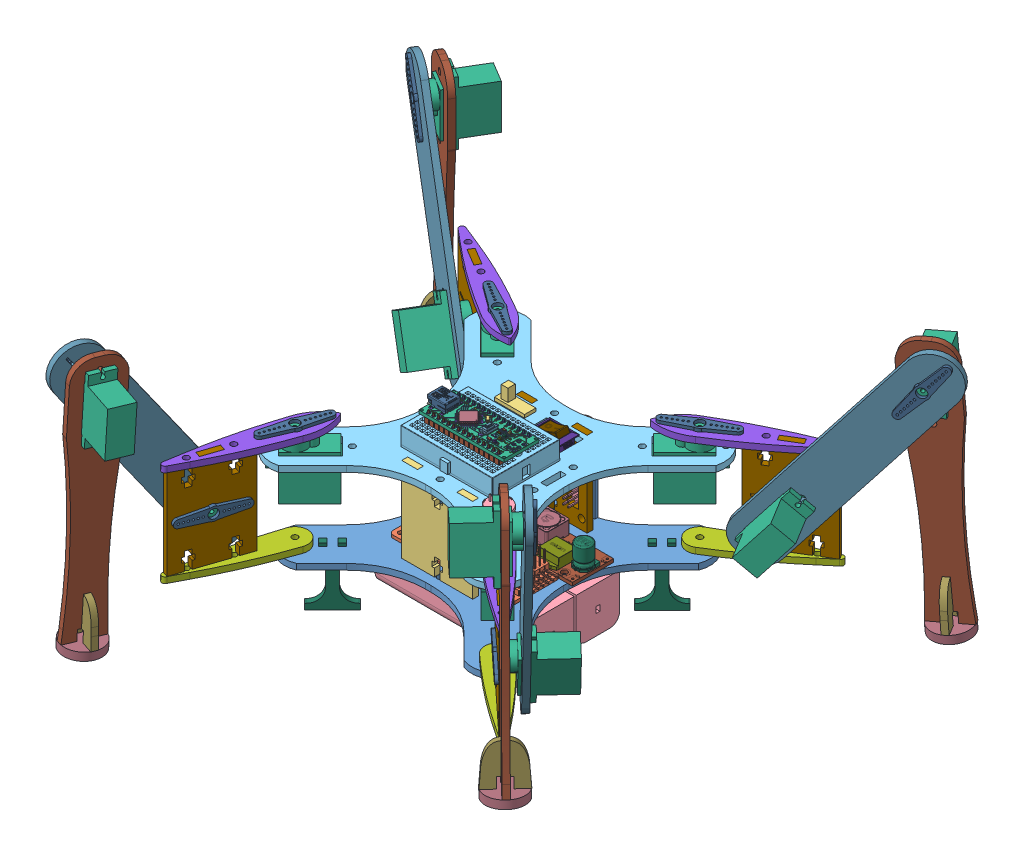
SolidWorks assembly SpiderBot_2_0, configuration Valor predeterminado. Lengths in mm. (continued)
Mates (geometry in assembly coordinates): (continued)
- Concêntrico12: concentric aligned: cylinder of Servo_knob2-6 through (379.7807 191.1423 -59.7062) axis (-0.507094 0 0.861891) radius 3.3; cylinder of Canela_mod-2 through (379.02 191.1423 -58.4134) axis (-0.507094 0 0.861891) radius 3.5
- Concêntrico13: concentric aligned: circle of Servo_knob2-6; circle of Servo-9
- Coincidente88: coincident anti-aligned: plane of Perna_baciadown-2 through (295.506 139.0953 -95.8306) normal (0 1 0); plane of Perna_coxa-2 through (317.9775 139.0953 -80.8691) normal (0 -1 0)
- Coincidente89: coincident anti-aligned: plane of Perna_baciadown-2 through (296.2666 139.0953 -97.1234) normal (-0.507094 0 0.861891); plane of Perna_coxa-2 through (310.018 161.5953 -89.0328) normal (0.507094 0 -0.861891)
- Coincidente90: coincident anti-aligned: plane of Perna_baciadown-2 through (313.5668 139.0953 -85.2045) normal (-0.861891 0 -0.507094); plane of Perna_coxa-2 through (312.8061 139.0953 -83.9116) normal (0.861891 0 0.507094)
- Coincidente91: coincident anti-aligned: plane of Servo-10 through (307.6949 160.7713 -90.7476) normal (-0.507094 0 0.861891); plane of Servo_knob2-7 through (310.1701 161.8953 -89.2913) normal (0.507094 0 -0.861891)
- Coincidente92: coincident anti-aligned: plane of Servo_knob2-7 through (308.4967 161.8953 -86.4471) normal (0.507094 0 -0.861891); plane of Perna_coxa-2 through (308.4967 161.5953 -86.4471) normal (-0.507094 0 0.861891)
- Coincidente93: coincident anti-aligned: plane of Pé_com_antiderrapante-2 through (374.0532 94.438 -47.8769) normal (-0.861885 0.003494 -0.507091); plane of comp_pé-2 through (371.6516 101.6677 -43.7453) normal (0.861885 -0.003494 0.507091)
- Coincidente94: coincident anti-aligned: plane of Servo_knob2-6 through (379.02 191.1423 -58.4134) normal (-0.507094 0 0.861891); plane of Canela_mod-2 through (376.9025 190.1943 -59.6593) normal (0.507094 0 -0.861891)
- Coincidente95: coincident anti-aligned: plane of Servo_knob2-6 through (377.3466 191.1423 -55.5692) normal (-0.507094 0 0.861891); plane of Servo-9 through (377.3373 188.0584 -55.5746) normal (0.507094 0 -0.861891)
- Coincidente96: coincident anti-aligned: plane of Pé_com_antiderrapante-2 through (376.3144 197.0356 -50.0272) normal (0.507094 0 -0.861891); plane of comp_pé-2 through (372.9888 94.4485 -51.9838) normal (-0.507094 0 0.861891)
- Bloquear6: lock: unknown of Servo_knob2-7; unknown of Perna_coxa-2
- Bloquear7: lock: unknown of Servo_knob2-6; unknown of Canela_mod-2
- Bloquear8: lock: unknown of comp_pé-2; unknown of Antiderrapante-2
- Coincidente97: coincident anti-aligned: plane of Canela_mod-2 through (376.9025 190.1943 -59.6593) normal (0.507094 0 -0.861891); plane of Servo-10 through (321.0332 171.2529 -92.53) normal (-0.507094 0 0.861891)
- Coincidente98: coincident anti-aligned: plane of Pé_com_antiderrapante-2 through (371.4675 94.4485 -49.3982) normal (-0.003012 -0.999994 -0.001772); plane of comp_pé-2 through (372.9888 94.4485 -51.9838) normal (0.003012 0.999994 0.001772)
- Coincidente99: coincident anti-aligned: plane of Pé_com_antiderrapante-2 through (371.4374 84.4485 -49.4159) normal (-0.003012 -0.999994 -0.001772); plane of Antiderrapante-2 through (373.5097 84.4432 -49.9236) normal (0.003012 0.999994 0.001772)
- Coincidente100: coincident anti-aligned: plane of Canela_mod-2 through (301.0832 155.7636 -104.2676) normal (0.802604 0.364474 0.472213); plane of Servo-10 through (297.0218 161.3392 -101.6681) normal (-0.802604 -0.364474 -0.472213)
- Coincidente101: coincident anti-aligned: plane of Canela_mod-2 through (375.0217 195.7698 -60.7659) normal (0.314137 -0.931214 0.184823); plane of Servo-10 through (315.0804 169.5398 -91.0433) normal (-0.314137 0.931214 -0.184823)
- Coincidente102: coincident anti-aligned: plane of Servo-9 through (380.4211 197.0216 -49.1193) normal (0.861885 -0.003494 0.507091); plane of Pé_com_antiderrapante-2 through (378.1729 174.5218 -45.4531) normal (-0.861885 0.003494 -0.507091)
- Coincidente103: coincident anti-aligned: plane of Servo-9 through (378.2548 201.7216 -45.4049) normal (0.507094 0 -0.861891); plane of Pé_com_antiderrapante-2 through (374.7931 197.0356 -47.4415) normal (-0.507094 0 0.861891)
- Coincidente104: coincident anti-aligned: plane of Servo-9 through (380.3534 174.5218 -49.1592) normal (-0.003012 -0.999994 -0.001772); plane of Pé_com_antiderrapante-2 through (378.1729 174.5218 -45.4531) normal (0.003012 0.999994 0.001772)
- Concêntrico14: concentric aligned: cylinder of Servo_knob2-10 through (40.3624 36.685 -2.4204) axis (-0.51295 0 0.858418) radius 3.3; cylinder of Perna_coxa-3 through (39.593 36.685 -1.1328) axis (-0.51295 0 0.858418) radius 3.5
- Concêntrico16: concentric aligned: circle of Servo-12; circle of Servo_knob2-10
- Concêntrico17: concentric aligned: cylinder of Servo_knob2-9 through (-6.1296 103.1368 -13.1938) axis (0.51295 0 -0.858418) radius 3.3; cylinder of Canela_mod-3 through (-5.3601 103.1368 -14.4815) axis (0.51295 0 -0.858418) radius 3.5
- Concêntrico18: concentric aligned: circle of Servo_knob2-9; circle of Servo-11
- Coincidente106: coincident anti-aligned: plane of Perna_baciaup-2 through (-71.7203 59.485 254.9925) normal (0 -1 0); plane of Perna_coxa-3 through (49.0356 59.485 4.5096) normal (0 1 0)
- Coincidente107: coincident anti-aligned: plane of Perna_baciaup-2 through (42.3462 62.485 4.0072) normal (0.51295 0 -0.858418); plane of Perna_coxa-3 through (38.0541 36.385 1.4424) normal (-0.51295 0 0.858418)
- Coincidente108: coincident anti-aligned: plane of Perna_baciaup-2 through (43.1157 62.485 2.7196) normal (-0.858418 0 -0.51295); plane of Perna_coxa-3 through (43.8851 62.485 1.4319) normal (0.858418 0 0.51295)
- Coincidente109: coincident anti-aligned: plane of Perna_baciadown-3 through (52.5195 13.885 8.3389) normal (0 1 0); plane of Perna_coxa-3 through (30.1504 13.885 -6.7753) normal (0 -1 0)
- Coincidente110: coincident anti-aligned: plane of Perna_baciadown-3 through (51.7501 13.885 9.6265) normal (0.51295 0 -0.858418); plane of Perna_coxa-3 through (38.0541 36.385 1.4424) normal (-0.51295 0 0.858418)
- Coincidente111: coincident anti-aligned: plane of Perna_baciadown-3 through (34.5315 13.885 -2.4099) normal (0.858418 0 0.51295); plane of Perna_coxa-3 through (35.3009 13.885 -3.6976) normal (-0.858418 0 -0.51295)
- Coincidente112: coincident anti-aligned: plane of Servo-12 through (39.3917 34.1371 2.5912) normal (0.51295 0 -0.858418); plane of Servo_knob2-10 through (37.9003 36.685 1.7) normal (-0.51295 0 0.858418)
- Coincidente113: coincident anti-aligned: plane of Servo_knob2-10 through (39.593 36.685 -1.1328) normal (-0.51295 0 0.858418); plane of Perna_coxa-3 through (39.593 36.385 -1.1328) normal (0.51295 0 -0.858418)
- Coincidente114: coincident anti-aligned: plane of Pé_com_antiderrapante-3 through (-0.7368 6.439 -25.232) normal (0.858417 -0.001507 0.51295); plane of comp_pé-3 through (1.7239 13.6688 -29.3286) normal (-0.858417 0.001507 -0.51295)
- Coincidente115: coincident anti-aligned: plane of Servo_knob2-9 through (-5.3601 103.1368 -14.4815) normal (0.51295 0 -0.858418); plane of Canela_mod-3 through (-4.0776 100.9682 -13.7151) normal (-0.51295 0 0.858418)
- Coincidente116: coincident anti-aligned: plane of Servo_knob2-9 through (-3.6674 103.1368 -17.3143) normal (0.51295 0 -0.858418); plane of Servo-11 through (-3.6714 100.0529 -17.3166) normal (-0.51295 0 0.858418)
- Coincidente117: coincident anti-aligned: plane of Pé_com_antiderrapante-3 through (340.7099 30.3509 182.2953) normal (-0.51295 0 0.858418); plane of comp_pé-3 through (0.2996 6.4345 -21.1179) normal (0.51295 0 -0.858418)
- Bloquear10: lock: unknown of Servo_knob2-10; unknown of Perna_coxa-3
- Bloquear11: lock: unknown of Servo_knob2-9; unknown of Canela_mod-3
- Bloquear12: lock: unknown of comp_pé-3; unknown of Antiderrapante-3
- Coincidente118: coincident anti-aligned: plane of Canela_mod-3 through (-4.0776 100.9682 -13.7151) normal (-0.51295 0 0.858418); plane of Servo-12 through (32.7007 48.7666 8.2619) normal (0.51295 0 -0.858418)
- Coincidente119: coincident anti-aligned: plane of Pé_com_antiderrapante-3 through (1.8385 6.4345 -23.6931) normal (-0.001293 -0.999999 -0.000773); plane of comp_pé-3 through (0.2996 6.4345 -21.1179) normal (0.001293 0.999999 0.000773)
- Coincidente120: coincident anti-aligned: plane of Pé_com_antiderrapante-3 through (3.2205 -3.5679 -22.8673) normal (-0.001293 -0.999999 -0.000773); plane of Antiderrapante-3 through (-0.2501 -3.5632 -23.2073) normal (0.001293 0.999999 0.000773)
- Coincidente121: coincident anti-aligned: plane of Canela_mod-3 through (41.609 22.921 13.5851) normal (-0.483627 0.826189 -0.288993); plane of Servo-12 through (48.061 26.2943 12.4313) normal (0.483627 -0.826189 0.288993)
- Coincidente122: coincident anti-aligned: plane of Canela_mod-3 through (0.1687 104.3415 -11.1777) normal (-0.709215 -0.563394 -0.423794); plane of Servo-12 through (37.1794 44.8835 5.929) normal (0.709215 0.563394 0.423794)
- Coincidente123: coincident anti-aligned: plane of Servo-11 through (-6.6726 109.0457 -23.7698) normal (-0.858417 0.001507 -0.51295); plane of Pé_com_antiderrapante-3 through (-4.4961 86.5457 -27.4784) normal (0.858417 -0.001507 0.51295)
- Coincidente124: coincident anti-aligned: plane of Servo-11 through (-4.4609 113.7457 -27.4573) normal (-0.51295 0 0.858418); plane of Pé_com_antiderrapante-3 through (342.2488 30.3509 179.72) normal (0.51295 0 -0.858418)
- Coincidente125: coincident anti-aligned: plane of Servo-11 through (-6.7017 86.5457 -23.7872) normal (-0.001293 -0.999999 -0.000773); plane of Pé_com_antiderrapante-3 through (-4.4961 86.5457 -27.4784) normal (0.001293 0.999999 0.000773)
- Concêntrico19: concentric aligned: cylinder of Servo-1 through (68.0098 62.385 17.5951) axis (0 -1 0) radius 2.3; cylinder of Servo_knob2-8 through (68.0098 63.985 17.5951) axis (0 -1 0) radius 2.3
- Coincidente126: coincident anti-aligned: plane of Servo-1 through (70.1904 59.185 19.7758) normal (0 1 0); plane of Servo_knob2-8 through (68.0098 59.185 17.5951) normal (0 -1 0)
- Concêntrico20: concentric aligned: cylinder of Perna_baciaup-2 through (68.0098 62.485 17.5951) axis (0 -1 0) radius 3.5; cylinder of Servo_knob2-8 through (68.0098 63.985 17.5951) axis (0 -1 0) radius 3.3
- Coincidente130: coincident anti-aligned: plane of Perna_baciaup-2 through (-71.7203 62.485 254.9925) normal (0 1 0); plane of Servo_knob2-8 through (68.0098 62.485 17.5951) normal (0 -1 0)
- Bloquear13: lock: unknown of Perna_baciaup-2; unknown of Servo_knob2-8
- Coincidente132: coincident anti-aligned: plane of Servo_knob2-12 through (67.8684 62.485 120.2635) normal (0 -1 0); plane of Perna_baciaup-3 through (329.6703 62.485 205.9477) normal (0 1 0)
- Concêntrico21: concentric anti-aligned: cylinder of Perna_coxa-4 through (55.6562 36.685 152.03) axis (0.94831 0 0.317345) radius 3.5; cylinder of Servo_knob2-11 through (59.9236 36.685 153.458) axis (-0.94831 0 -0.317345) radius 3.3
- Concêntrico22: concentric aligned: circle of Servo_knob2-12; circle of Perna_baciaup-3
- Bloquear14: lock: unknown of Servo_knob2-12; unknown of Perna_baciaup-3
- Coincidente133: coincident anti-aligned: plane of Perna_coxa-4 through (59.147 59.485 141.5986) normal (0 1 0); plane of Perna_baciaup-3 through (329.6703 59.485 205.9477) normal (0 -1 0)
- Coincidente134: coincident anti-aligned: plane of Perna_coxa-4 through (58.5011 36.385 152.982) normal (0.94831 0 0.317345); plane of Perna_baciaup-3 through (60.0878 62.485 148.2405) normal (-0.94831 0 -0.317345)
- Coincidente135: coincident anti-aligned: plane of Perna_coxa-4 through (57.2429 62.485 147.2884) normal (0.317345 0 -0.94831); plane of Perna_baciaup-3 through (58.6654 62.485 147.7645) normal (-0.317345 0 0.94831)
- Coincidente136: coincident anti-aligned: plane of Perna_coxa-4 through (52.1654 13.885 162.4614) normal (0 -1 0); plane of Perna_baciadown-4 through (62.1418 13.885 137.3758) normal (0 1 0)
- Coincidente138: coincident anti-aligned: plane of Perna_coxa-4 through (54.0695 13.885 156.7715) normal (-0.317345 0 0.94831); plane of Perna_baciadown-4 through (55.4919 13.885 157.2476) normal (0.317345 0 -0.94831)
- Concêntrico23: concentric aligned: cylinder of Servo-4 through (67.8684 62.385 120.2635) axis (0 -1 0) radius 2.3; cylinder of Servo_knob2-12 through (67.8684 63.985 120.2635) axis (0 -1 0) radius 2.3
- Coincidente140: coincident anti-aligned: plane of Servo-4 through (70.049 59.185 118.0828) normal (0 1 0); plane of Servo_knob2-12 through (67.8684 59.185 120.2635) normal (0 -1 0)
- Coincidente141: coincident anti-aligned: plane of Perna_coxa-4 through (58.5011 36.385 152.982) normal (0.94831 0 0.317345); plane of Servo_knob2-11 through (58.5011 36.685 152.982) normal (-0.94831 0 -0.317345)
- Bloquear16: lock: unknown of Perna_coxa-4; unknown of Servo_knob2-11
- Concêntrico24: concentric aligned: cylinder of Servo_knob2-13 through (31.6845 103.1908 191.837) axis (0.94831 0 0.317345) radius 3.3; cylinder of Canela_mod-4 through (33.107 103.1908 192.3131) axis (0.94831 0 0.317345) radius 3.5
- Concêntrico25: concentric aligned: circle of Servo_knob2-13; circle of Servo-13
- Coincidente143: coincident anti-aligned: plane of Pé_com_antiderrapante-4 through (42.9446 6.5501 199.469) normal (-0.31691 0.05235 0.94701); plane of comp_pé-4 through (47.5965 13.7699 200.6266) normal (0.31691 -0.05235 -0.94701)
- Coincidente144: coincident anti-aligned: plane of Servo_knob2-13 through (33.107 103.1908 192.3131) normal (0.94831 0 0.317345); plane of Canela_mod-4 through (33.5754 101.0099 190.9133) normal (-0.94831 0 -0.317345)
- Coincidente145: coincident anti-aligned: plane of Servo_knob2-13 through (36.2364 103.1908 193.3603) normal (0.94831 0 0.317345); plane of Servo-13 through (36.1852 100.1111 193.5134) normal (-0.94831 0 -0.317345)
- Coincidente146: coincident anti-aligned: plane of Pé_com_antiderrapante-4 through (-86.1045 51.945 575.6482) normal (-0.94831 0 -0.317345); plane of comp_pé-4 through (39.1489 6.7072 201.358) normal (0.94831 0 0.317345)
- Bloquear17: lock: unknown of Servo_knob2-13; unknown of Canela_mod-4
- Bloquear18: lock: unknown of comp_pé-4; unknown of Antiderrapante-4
- Coincidente147: coincident anti-aligned: plane of Canela_mod-4 through (33.5754 101.0099 190.9133) normal (-0.94831 0 -0.317345); plane of Servo-14 through (44.0564 42.1045 159.5933) normal (0.94831 0 0.317345)
- Coincidente148: coincident anti-aligned: plane of Pé_com_antiderrapante-4 through (41.9939 6.7072 202.31) normal (-0.016613 -0.998629 0.049644); plane of comp_pé-4 through (39.1489 6.7072 201.358) normal (0.016613 0.998629 -0.049644)
- Coincidente149: coincident anti-aligned: plane of Pé_com_antiderrapante-4 through (41.3128 -3.1941 204.3454) normal (-0.016613 -0.998629 0.049644); plane of Antiderrapante-4 through (40.9007 -3.3591 200.8865) normal (0.016613 0.998629 -0.049644)
- Coincidente150: coincident anti-aligned: plane of Canela_mod-4 through (50.4972 23.0317 140.3467) normal (-0.179129 0.825458 0.535286); plane of Servo-14 through (53.0065 19.652 146.3981) normal (0.179129 -0.825458 -0.535286)
- Coincidente151: coincident anti-aligned: plane of Canela_mod-4 through (32.007 97.6303 195.6002) normal (0.261955 0.564463 -0.782791); plane of Servo-14 through (48.9761 38.2248 158.4421) normal (-0.261955 -0.564463 0.782791)
- Coincidente152: coincident anti-aligned: plane of Servo-13 through (41.9974 108.7739 188.7494) normal (0.31691 -0.05235 -0.94701); plane of Pé_com_antiderrapante-4 through (45.7014 86.3047 191.231) normal (-0.31691 0.05235 0.94701)
- Coincidente153: coincident anti-aligned: plane of Servo-13 through (46.1533 113.4674 189.8807) normal (-0.94831 0 -0.317345); plane of Pé_com_antiderrapante-4 through (-83.2595 51.945 576.6003) normal (0.94831 0 0.317345)
- Coincidente154: coincident anti-aligned: plane of Servo-13 through (41.6237 86.3047 189.8664) normal (-0.016613 -0.998629 0.049644); plane of Pé_com_antiderrapante-4 through (45.7014 86.3047 191.231) normal (0.016613 0.998629 -0.049644)
- Concêntrico26: concentric aligned: cylinder of Servo_knob2-11 through (59.9236 36.685 153.458) axis (-0.94831 0 -0.317345) radius 2.3; cylinder of Servo-14 through (58.4063 36.685 152.9503) axis (-0.94831 0 -0.317345) radius 2.3
- Coincidente155: coincident anti-aligned: plane of Servo_knob2-11 through (55.3717 36.685 151.9348) normal (-0.94831 0 -0.317345); plane of Servo-14 through (55.9241 34.1393 150.284) normal (0.94831 0 0.317345)
- Coincidente157: coincident anti-aligned: plane of Perna_coxa-4 through (55.6562 36.385 152.03) normal (-0.94831 0 -0.317345); plane of Perna_baciadown-4 through (60.7194 13.885 136.8998) normal (0.94831 0 0.317345)
- Concêntrico27: concentric aligned: circle of Servo-15; circle of Servo_knob2-16
- Concêntrico28: concentric aligned: cylinder of Canela_mod-5 through (211.9581 132.8204 185.1709) axis (0.612502 0 0.790469) radius 3.5; cylinder of Servo_knob2-16 through (211.0394 132.8204 183.9852) axis (0.612502 0 0.790469) radius 3.3
- Bloquear19: lock: unknown of Servo_knob2-15; unknown of Perna_coxa-5
- Bloquear20: lock: unknown of Canela_mod-5; unknown of Servo_knob2-16
- Bloquear21: lock: unknown of Antiderrapante-5; unknown of comp_pé-5
- Concêntrico29: concentric anti-aligned: cylinder of Servo_knob2-15 through (272.6999 87.7379 154.677) axis (-0.612502 0 -0.790469) radius 3.3; cylinder of Perna_coxa-5 through (269.9436 87.7379 151.1199) axis (0.612502 0 0.790469) radius 3.5
- Coincidente158: coincident anti-aligned: plane of Perna_baciadown-5 through (282.5555 64.9379 141.3475) normal (0.612502 0 0.790469); plane of Perna_coxa-5 through (269.9436 87.4379 151.1199) normal (-0.612502 0 -0.790469)
- Coincidente159: coincident anti-aligned: plane of Perna_baciadown-5 through (283.4742 64.9379 142.5332) normal (0 1 0); plane of Perna_coxa-5 through (261.2485 64.9379 157.8575) normal (0 -1 0)
- Coincidente160: coincident anti-aligned: plane of Perna_baciaup-4 through (275.7335 113.5379 150.4288) normal (-0.612502 0 -0.790469); plane of Perna_coxa-5 through (271.7812 87.4379 153.4913) normal (0.612502 0 0.790469)
- Coincidente162: coincident anti-aligned: plane of Perna_baciaup-4 through (467.9023 110.5379 348.1053) normal (0 -1 0); plane of Perna_coxa-5 through (278.6388 110.5379 144.3824) normal (0 1 0)
- Coincidente163: coincident anti-aligned: plane of Perna_baciadown-5 through (266.9101 64.9379 155.3681) normal (0.790469 0 -0.612502); plane of Perna_coxa-5 through (265.9913 64.9379 154.1824) normal (-0.790469 0 0.612502)
- Coincidente164: coincident anti-aligned: plane of Perna_baciaup-4 through (274.8147 113.5379 149.2431) normal (-0.790469 0 0.612502); plane of Perna_coxa-5 through (273.896 113.5379 148.0574) normal (0.790469 0 -0.612502)
- Coincidente165: coincident anti-aligned: plane of Servo-15 through (225.8361 141.4085 189.0923) normal (-0.612502 0 -0.790469); plane of Pé_com_antiderrapante-5 through (221.7805 137.9782 192.2348) normal (0.612502 0 0.790469)
- Coincidente166: coincident anti-aligned: plane of comp_pé-5 through (203.7589 46.3626 212.2445) normal (0.760479 -0.272836 -0.589264); plane of Pé_com_antiderrapante-5 through (199.2727 39.4072 209.6752) normal (-0.760479 0.272836 0.589264)
- Coincidente167: coincident anti-aligned: plane of Servo-15 through (213.3143 129.8535 188.2948) normal (-0.612502 0 -0.790469); plane of Servo_knob2-16 through (213.9794 132.8204 187.7795) normal (0.612502 0 0.790469)
- Coincidente168: coincident anti-aligned: plane of comp_pé-5 through (195.1537 40.2257 209.0716) normal (0.612502 0 0.790469); plane of Pé_com_antiderrapante-5 through (219.943 137.9782 189.8634) normal (-0.612502 0 -0.790469)
- Coincidente169: coincident anti-aligned: plane of comp_pé-5 through (195.1537 40.2257 209.0716) normal (0.215669 0.96206 -0.167113); plane of Pé_com_antiderrapante-5 through (196.9912 40.2257 211.443) normal (-0.215669 -0.96206 0.167113)
- Coincidente170: coincident anti-aligned: plane of Antiderrapante-5 through (195.0854 30.188 211.0368) normal (0.215669 0.96206 -0.167113); plane of Pé_com_antiderrapante-5 through (194.8345 30.6051 213.1141) normal (-0.215669 -0.96206 0.167113)
- Coincidente171: coincident anti-aligned: plane of Servo-15 through (222.1887 136.8868 186.4787) normal (0.760479 -0.272836 -0.589264); plane of Pé_com_antiderrapante-5 through (219.9699 115.2405 193.6378) normal (-0.760479 0.272836 0.589264)
- Coincidente172: coincident anti-aligned: plane of Canela_mod-5 through (213.6786 131.3379 183.8378) normal (-0.612502 0 -0.790469); plane of Servo_knob2-16 through (211.9581 132.8204 185.1709) normal (0.612502 0 0.790469)
- Coincidente173: coincident anti-aligned: plane of Servo-15 through (217.3361 115.2405 190.2388) normal (-0.215669 -0.96206 0.167113); plane of Pé_com_antiderrapante-5 through (219.9699 115.2405 193.6378) normal (0.215669 0.96206 -0.167113)
- Coincidente174: coincident anti-aligned: plane of Servo_knob2-15 through (271.7812 87.7379 153.4913) normal (-0.612502 0 -0.790469); plane of Perna_coxa-5 through (271.7812 87.4379 153.4913) normal (0.612502 0 0.790469)
- Concêntrico31: concentric aligned: cylinder of Servo-17 through (198.857 36.685 -1.2707) axis (0.519699 0 0.85435) radius 2.3; cylinder of Servo_knob2-17 through (198.0255 36.685 -2.6377) axis (0.519699 0 0.85435) radius 2.3
- Concêntrico32: concentric aligned: circle of Servo-16; circle of Servo_knob2-18
- Concêntrico33: concentric aligned: cylinder of Canela_mod-6 through (248.1937 99.1708 -17.8216) axis (-0.519699 0 -0.85435) radius 3.5; cylinder of Servo_knob2-18 through (248.9732 99.1708 -16.54) axis (-0.519699 0 -0.85435) radius 3.3
- Bloquear23: lock: unknown of Servo_knob2-17; unknown of Perna_coxa-6
- Bloquear24: lock: unknown of Canela_mod-6; unknown of Servo_knob2-18
- Concêntrico34: concentric anti-aligned: cylinder of Servo_knob2-17 through (198.0255 36.685 -2.6377) axis (0.519699 0 0.85435) radius 3.3; cylinder of Perna_coxa-6 through (200.3641 36.685 1.2069) axis (-0.519699 0 -0.85435) radius 3.5
- Concêntrico35: concentric aligned: circle of Servo_knob2-19; circle of Perna_baciaup-5
- Bloquear26: lock: unknown of Servo_knob2-19; unknown of Perna_baciaup-5
- Coincidente175: coincident anti-aligned: plane of Servo-17 through (198.8564 34.2936 2.4752) normal (-0.519699 0 -0.85435); plane of Servo_knob2-17 through (200.52 36.685 1.4632) normal (0.519699 0 0.85435)
- Coincidente176: coincident anti-aligned: plane of Perna_baciadown-6 through (186.7331 13.885 9.4986) normal (-0.519699 0 -0.85435); plane of Perna_coxa-6 through (200.3641 36.385 1.2069) normal (0.519699 0 0.85435)
- Coincidente177: coincident anti-aligned: plane of Perna_baciadown-6 through (185.9535 13.885 8.2171) normal (0 1 0); plane of Perna_coxa-6 through (209.762 13.885 -4.5098) normal (0 -1 0)
- Coincidente178: coincident anti-aligned: plane of Perna_baciaup-5 through (194.5333 62.485 1.2423) normal (0.519699 0 0.85435); plane of Perna_coxa-6 through (198.805 36.385 -1.3562) normal (-0.519699 0 -0.85435)
- Coincidente179: coincident anti-aligned: plane of Servo_knob2-19 through (170.5367 62.485 17.5951) normal (0 -1 0); plane of Perna_baciaup-5 through (25.8198 62.485 -216.7957) normal (0 1 0)
- Coincidente180: coincident anti-aligned: plane of Perna_baciaup-5 through (25.8198 59.485 -216.7957) normal (0 -1 0); plane of Perna_coxa-6 through (190.9663 59.485 6.9236) normal (0 1 0)
- Coincidente181: coincident anti-aligned: plane of Perna_baciadown-6 through (203.8563 13.885 -2.6731) normal (-0.85435 0 0.519699); plane of Perna_coxa-6 through (204.6359 13.885 -1.3916) normal (0.85435 0 -0.519699)
- Coincidente182: coincident anti-aligned: plane of Perna_baciaup-5 through (195.3128 62.485 2.5239) normal (0.85435 0 -0.519699); plane of Perna_coxa-6 through (196.0924 62.485 3.8054) normal (-0.85435 0 0.519699)
- Coincidente183: coincident anti-aligned: plane of Servo-16 through (236.4603 109.299 -24.2618) normal (0.519699 0 0.85435); plane of Pé_com_antiderrapante-6 through (585.9618 57.0093 -236.8627) normal (-0.519699 0 -0.85435)
- Coincidente184: coincident anti-aligned: plane of comp_pé-6 through (244.2147 9.847 -34.5723) normal (-0.851949 -0.074907 0.518239); plane of Pé_com_antiderrapante-6 through (247.1609 2.6376 -30.7709) normal (0.851949 0.074907 -0.518239)
- Coincidente185: coincident anti-aligned: plane of Servo-16 through (246.676 96.0955 -20.761) normal (0.519699 0 0.85435); plane of Servo_knob2-18 through (246.4787 99.1708 -20.6409) normal (-0.519699 0 -0.85435)
- Coincidente186: coincident anti-aligned: plane of comp_pé-6 through (251.2759 2.8623 -29.7626) normal (-0.519699 0 -0.85435); plane of Pé_com_antiderrapante-6 through (587.5209 57.0093 -234.2997) normal (0.519699 0 0.85435)
- Coincidente187: coincident anti-aligned: plane of Servo-17 through (214.4605 41.1792 2.6982) normal (-0.519699 0 -0.85435); plane of Canela_mod-6 through (246.7814 97.1208 -16.9625) normal (0.519699 0 0.85435)
- Coincidente188: coincident anti-aligned: plane of comp_pé-6 through (251.2759 2.8623 -29.7626) normal (-0.063997 0.997191 0.038929); plane of Pé_com_antiderrapante-6 through (249.7168 2.8623 -32.3256) normal (0.063997 -0.997191 -0.038929)
- Coincidente190: coincident anti-aligned: plane of Servo-17 through (197.5526 20.0873 7.9502) normal (-0.539458 -0.775437 0.328151); plane of Canela_mod-6 through (195.8207 23.8679 14.0368) normal (0.539458 0.775437 -0.328151)
- Coincidente191: coincident anti-aligned: plane of Servo-17 through (209.6904 37.5346 0.5668) normal (0.662494 -0.631425 -0.402994); plane of Canela_mod-6 through (250.748 93.3402 -19.3754) normal (-0.662494 0.631425 0.402994)
- Coincidente192: coincident anti-aligned: plane of Servo-16 through (238.9958 104.6122 -20.771) normal (-0.851949 -0.074907 0.518239); plane of Pé_com_antiderrapante-6 through (238.201 82.1754 -25.3206) normal (0.851949 0.074907 -0.518239)
- Coincidente193: coincident anti-aligned: plane of Canela_mod-6 through (246.7814 97.1208 -16.9625) normal (0.519699 0 0.85435); plane of Servo_knob2-18 through (248.1937 99.1708 -17.8216) normal (-0.519699 0 -0.85435)
- Coincidente194: coincident anti-aligned: plane of Servo-16 through (240.4357 82.1754 -21.6469) normal (0.063997 -0.997191 -0.038929); plane of Pé_com_antiderrapante-6 through (238.201 82.1754 -25.3206) normal (-0.063997 0.997191 0.038929)
- Coincidente195: coincident anti-aligned: plane of Servo_knob2-17 through (198.805 36.685 -1.3562) normal (0.519699 0 0.85435); plane of Perna_coxa-6 through (198.805 36.385 -1.3562) normal (-0.519699 0 -0.85435)
- Concêntrico36: concentric aligned: cylinder of Servo-2 through (170.5367 62.385 17.5951) axis (0 -1 0) radius 2.3; cylinder of Servo_knob2-19 through (170.5367 63.985 17.5951) axis (0 -1 0) radius 2.3
- Coincidente196: coincident anti-aligned: plane of Servo-2 through (168.3561 59.185 19.7758) normal (0 1 0); plane of Servo_knob2-19 through (170.5367 59.185 17.5951) normal (0 -1 0)
- Coincidente197: coincident anti-aligned: plane of base-1 through (23.9756 10.885 83.5502) normal (0.707107 0 0.707107); plane of suporte_embaixo-1 through (77.776 7.885 29.7498) normal (-0.707107 0 -0.707107)
- Coincidente198: coincident anti-aligned: plane of base-1 through (63.3472 10.885 11.0783) normal (-0.707107 0 0.707107); plane of suporte_embaixo-1 through (78.2165 7.8091 25.9476) normal (0.707107 0 -0.707107)
- Coincidente199: coincident anti-aligned: plane of base-1 through (7.4255 7.885 67) normal (0 -1 0); plane of suporte_embaixo-1 through (74.9476 7.885 26.9214) normal (0 1 0)
- Coincidente200: coincident anti-aligned: plane of base-1 through (61.3516 10.885 13.0739) normal (0.707107 0 -0.707107); plane of suporte_embaixo-3 through (159.7968 7.8091 111.5191) normal (-0.707107 0 0.707107)
- Coincidente201: coincident anti-aligned: plane of base-1 through (102.6018 10.885 162.1763) normal (0.707107 0 0.707107); plane of suporte_embaixo-3 through (156.5279 7.885 108.2502) normal (-0.707107 0 -0.707107)
- Coincidente202: coincident anti-aligned: plane of base-1 through (7.4255 7.885 67) normal (0 -1 0); plane of suporte_embaixo-3 through (158.6492 7.885 110.3715) normal (0 1 0)
- Coincidente203: coincident anti-aligned: plane of base-1 through (100.6018 10.885 -26.1763) normal (0.707107 0 -0.707107); plane of suporte_embaixo-2 through (158.6492 7.885 31.8711) normal (-0.707107 0 0.707107)
- Coincidente204: coincident anti-aligned: plane of base-1 through (63.3516 10.885 122.9261) normal (0.707107 0 0.707107); plane of suporte_embaixo-2 through (159.7968 7.8091 26.4809) normal (-0.707107 0 -0.707107)
- Coincidente205: coincident anti-aligned: plane of base-1 through (7.4255 7.885 67) normal (0 -1 0); plane of suporte_embaixo-2 through (160.7705 7.885 29.7498) normal (0 1 0)
- Coincidente206: coincident anti-aligned: plane of base-1 through (65.3472 10.885 124.9217) normal (-0.707107 0 -0.707107); plane of suporte_embaixo-4 through (78.7497 7.8091 111.5191) normal (0.707107 0 0.707107)
- Coincidente207: coincident anti-aligned: plane of base-1 through (24.0969 10.885 50.3285) normal (-0.707107 0 0.707107); plane of suporte_embaixo-4 through (79.8973 7.885 106.1289) normal (0.707107 0 -0.707107)
- Coincidente208: coincident anti-aligned: plane of base-1 through (7.4255 7.885 67) normal (0 -1 0); plane of suporte_embaixo-4 through (77.776 7.885 108.2502) normal (0 1 0)
- Concêntrico38: concentric aligned: cylinder of base-1 through (132.2732 10.885 80.5) axis (0 -1 0) radius 1.5; cylinder of Bateria-1 through (132.2732 7.885 80.5) axis (0 -1 0) radius 1.5
- Concêntrico39: concentric aligned: cylinder of base-1 through (106.2732 10.885 80.5) axis (0 -1 0) radius 1.5; cylinder of Bateria-1 through (106.2732 7.885 80.5) axis (0 -1 0) radius 1.5
- Concêntrico40: concentric aligned: cylinder of base-1 through (132.2732 10.885 57.5) axis (0 -1 0) radius 1.5; cylinder of Bateria-3 through (132.2732 7.885 57.5) axis (0 -1 0) radius 1.5
- Concêntrico41: concentric aligned: cylinder of base-1 through (106.2732 10.885 57.5) axis (0 -1 0) radius 1.5; cylinder of Bateria-3 through (106.2732 7.885 57.5) axis (0 -1 0) radius 1.5
- Coincidente211: coincident anti-aligned: plane of base-1 through (7.4255 7.885 67) normal (0 -1 0); plane of Bateria-1 through (79.7732 7.885 80.5) normal (0 1 0)
- Coincidente212: coincident anti-aligned: plane of base-1 through (7.4255 7.885 67) normal (0 -1 0); plane of Bateria-3 through (79.7732 7.885 57.5) normal (0 1 0)
- Paralelo13: parallel anti-aligned: plane of suporte_mod_cam-1 through (123.0232 10.885 41.5) normal (0 0 1); plane of LM2596 DC-DC StepDown Converter v1.step-1/Trimpot 3296W v1.step-1 through (128.3132 12.485 62.47) normal (0 0 -1)
- Coincidente214: coincident anti-aligned: plane of base-1 through (7.4255 10.885 67) normal (0 1 0); plane of LM2596 DC-DC StepDown Converter v1.step-1/Board v5.step-1 through (135.2732 10.885 58) normal (0 -1 0)
- Concêntrico42: concentric anti-aligned: cylinder of base-1 through (120.2732 10.885 50) axis (0 -1 0) radius 1.5; cylinder of LM2596 DC-DC StepDown Converter v1.step-1/Board v5.step-1 through (120.2732 10.885 50) axis (0 1 0) radius 1.5
- Concêntrico43: concentric anti-aligned: cylinder of base-1 through (91.2732 10.885 71) axis (0 -1 0) radius 1.25; cylinder of PCA9685-1 through (91.2732 10.885 71) axis (0 1 0) radius 1.25
- Concêntrico44: concentric anti-aligned: cylinder of base-1 through (147.2732 10.885 90) axis (0 -1 0) radius 1.25; cylinder of PCA9685-1 through (147.2732 10.885 90) axis (0 1 0) radius 1.25
- Coincidente215: coincident anti-aligned: plane of base-1 through (7.4255 10.885 67) normal (0 1 0); plane of PCA9685-1 through (88.2732 10.885 93) normal (0 -1 0)
- Concêntrico49: concentric anti-aligned: cylinder of base_cima-1 through (124.7732 53.885 76) axis (0 -1 0) radius 1.5; cylinder of Placa_GY521-1 through (124.7732 49.885 76) axis (0 1 0) radius 1.5875
- Coincidente217: coincident anti-aligned: plane of base_cima-1 through (7.4255 50.885 67) normal (0 -1 0); plane of Placa_GY521-1 through (118.6183 50.885 67.7208) normal (0 1 0)
- Coincidente218: coincident anti-aligned: plane of base_cima-1 through (7.4255 53.885 44.0553) normal (0 0 1); plane of switch_pequeno-1 through (98.5232 49.3004 44.0553) normal (0 0 -1)
- Coincidente219: coincident anti-aligned: plane of base_cima-1 through (98.5232 53.885 67) normal (1 0 0); plane of switch_pequeno-1 through (98.5232 49.3004 49.8053) normal (-1 0 0)
- Concêntrico52: concentric aligned: cylinder of base_cima-1 through (149.0184 53.885 98) axis (0 -1 0) radius 5.85; cylinder of Buzzer_Active.stp-1 through (149.0184 57.9073 98) axis (0 -1 0) radius 5.925
- Concêntrico53: concentric anti-aligned: cylinder of base-1 through (94.5547 10.885 43.1958) axis (0 -1 0) radius 2.5; cylinder of LED-2 through (94.5547 3.285 43.1958) axis (0 1 0) radius 2.5
- Coincidente220: coincident aligned: plane of base-1 through (7.4255 10.885 67) normal (0 1 0); circle of LED-2
- Concêntrico54: concentric anti-aligned: cylinder of base-1 through (88.3285 10.885 43.1958) axis (0 -1 0) radius 2.5; cylinder of LED-1 through (88.3285 3.285 43.1958) axis (0 1 0) radius 2.5
- Coincidente221: coincident anti-aligned: plane of base-1 through (7.4255 10.885 67) normal (0 1 0); plane of LED-1 through (88.3285 10.885 43.1958) normal (0 -1 0)
- Coincidente225: coincident anti-aligned: plane of Pé_com_antiderrapante-6 through (251.7412 -6.9879 -33.5571) normal (0.063997 -0.997191 -0.038929); plane of Antiderrapante-7 through (249.6898 -7.2369 -30.5498) normal (-0.063997 0.997191 0.038929)
- Bloquear27: lock: unknown of comp_pé-6; unknown of Antiderrapante-7
